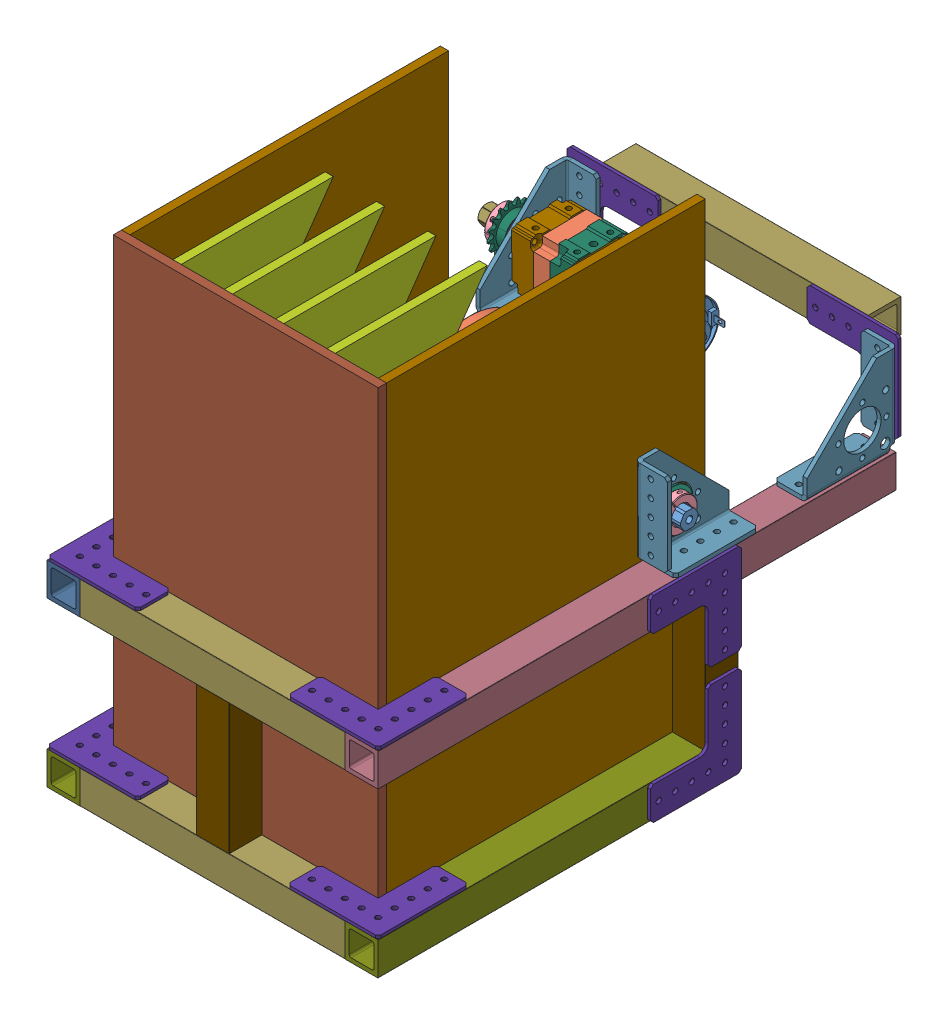
SolidWorks assembly Assem_Launch_Component(wheels,hexshaft,motor,etc.)-SP - Copy, configuration Default. Lengths in mm.
Overall size (290.76 381 426.56).
90 component instances, 36 part files, 140 mates.
Components (placement in the parent):
- ThunderHex(.5 11inch)-SP-1: ThunderHex(.5 11inch)-SP [Default] at (-34.4752 190.5 -222.25) x (0 0.015634 -0.999878) z (-1 0 0) size (13.74 12.75 279.4)
- CompliantWheel(4inch 500)SP-1: CompliantWheel(4inch 500)SP [Default] at (-57.548 185.9668 -238.3103) x (0 -0.486399 -0.873737) z (-1 0 0) size (101.6 101.6 25.4)
  - CompliantWheel(4inch 500)SP.STEP-1: CompliantWheel(4inch 500)SP.STEP [Default] at origin size (101.6 101.6 25.4)
    - 4IN Compliant Wheel FINAL Overmold.STEP-1: 4IN Compliant Wheel FINAL Overmold.STEP [Default] at (-16.2374 3.8509 18.652) size (101.6 101.6 25.4)
    - 2in Wheel Intergrated 0500 HEX Hub.STEP-1: 2in Wheel Intergrated 0500 HEX Hub.STEP [Default] at (-16.2374 3.8509 5.952) x (-1 0 0) z (0 0 -1) size (41.91 41.91 25.4)
- CompliantWheel(4inch 500)SP.STEP-1: CompliantWheel(4inch 500)SP.STEP [Default] at (-82.948 195.0332 -206.1897) x (0 0.486399 0.873737) z (-1 0 0) size (101.6 101.6 25.4)
  - 4IN Compliant Wheel FINAL Overmold.STEP-1: 4IN Compliant Wheel FINAL Overmold.STEP [Default] at (-16.2374 3.8509 18.652) size (101.6 101.6 25.4)
  - 2in Wheel Intergrated 0500 HEX Hub.STEP-1: 2in Wheel Intergrated 0500 HEX Hub.STEP [Default] at (-16.2374 3.8509 5.952) x (-1 0 0) z (0 0 -1) size (41.91 41.91 25.4)
- CompliantWheel(4inch 500)SP.STEP-3: CompliantWheel(4inch 500)SP.STEP [Default] at (-108.348 195.2838 -206.2625) x (0 0.5 0.866025) z (-1 0 0) size (101.6 101.6 25.4)
  - 4IN Compliant Wheel FINAL Overmold.STEP-1: 4IN Compliant Wheel FINAL Overmold.STEP [Default] at (-16.2374 3.8509 18.652) size (101.6 101.6 25.4)
  - 2in Wheel Intergrated 0500 HEX Hub.STEP-1: 2in Wheel Intergrated 0500 HEX Hub.STEP [Default] at (-16.2374 3.8509 5.952) x (-1 0 0) z (0 0 -1) size (41.91 41.91 25.4)
- CompliantWheel(4inch 500)SP.STEP-4: CompliantWheel(4inch 500)SP.STEP [Default] at (-133.748 195.0332 -206.1897) x (0 0.486399 0.873737) z (-1 0 0) size (101.6 101.6 25.4)
  - 4IN Compliant Wheel FINAL Overmold.STEP-1: 4IN Compliant Wheel FINAL Overmold.STEP [Default] at (-16.2374 3.8509 18.652) size (101.6 101.6 25.4)
  - 2in Wheel Intergrated 0500 HEX Hub.STEP-1: 2in Wheel Intergrated 0500 HEX Hub.STEP [Default] at (-16.2374 3.8509 5.952) x (-1 0 0) z (0 0 -1) size (41.91 41.91 25.4)
- ClampingShaftCollar(.5 in)SP-1: ClampingShaftCollar(.5 in)SP [Default] at (-47.625 190.7032 -222.2468) x (0 0.015634 -0.999878) z (-1 0 0) size (25.39 25.4 6.35)
- ClampingShaftCollar(.5 in)SP-2: ClampingShaftCollar(.5 in)SP [Default] at (-155.575 190.4012 -222.4275) x (0 0.873737 -0.486399) z (-1 0 0) size (25.39 25.4 6.35)
- VersaPlanetaryv2_Single_Stage_10_1_with_775_Series (General_GearBox_Shell)-SP-1: VersaPlanetaryv2_Single_Stage_10_1_with_775_Series (General_GearBox_Shell)-SP [Default] at (-205.875 214.6824 -345.637) x (-1 0 0) z (0 -0.015634 0.999878) size (166.6 51.28 52.65)
  - VersaPlanetary_v2_Single_Stage_10_1_with_775_Series (General_GearBox_Shell)-SP.STEP-1: VersaPlanetary_v2_Single_Stage_10_1_with_775_Series (General_GearBox_Shell)-SP.STEP [Default] at origin size (166.6 51.28 52.65)
    - 217-2820 Rev1_Public.STEP-1: 217-2820 Rev1_Public.STEP [Default] at (-4.6546 22.225 0) x (0 -0.456494 0.889726) z (-1 0 0) size (39.22 38.88 17.4)
      - 217-2625-100.STEP-1: 217-2625-100.STEP [Default] at origin size (39.22 38.88 12.7)
        - 217-2625-008 Rev1.STEP-1: 217-2625-008 Rev1.STEP [Default] at origin size (34.7 34.7 4.7)
        - 217-2625-010 Rev1.STEP-1: 217-2625-010 Rev1.STEP [Default] at (0 10.193 3.65) x (0.999813 0.019336 0) z (0 0 1) size (4 4 12)
        - 217-2625-010 Rev1.STEP-2: 217-2625-010 Rev1.STEP [Default] at (8.691 -5.3258 3.65) size (4 4 12)
        - 217-2625-010 Rev1.STEP-3: 217-2625-010 Rev1.STEP [Default] at (-8.691 -5.3258 3.65) size (4 4 12)
        - 217-2625-005 Rev1_Planet_Revolving_Follower01.STEP-1: 217-2625-005 Rev1_Planet_Revolving_Follower01.STEP [Default] at (8.691 -5.3258 6.35) x (0.932816 0.360354 0) z (0 0 1) size (16.89 16.89 8)
        - 217-2625-005 Rev1_Planet_Revolving_Follower01.STEP-2: 217-2625-005 Rev1_Planet_Revolving_Follower01.STEP [Default] at (-8.691 -5.3258 6.35) x (-0.932788 -0.360426 0) z (0 0 1) size (16.89 16.89 8)
        - 217-2625-005 Rev1_Planet_Revolving_Follower01.STEP-3: 217-2625-005 Rev1_Planet_Revolving_Follower01.STEP [Default] at (0 10.193 6.35) x (0.893583 0.448898 0) z (0 0 1) size (16.89 16.89 8)
      - 217-2625-007 Rev1_Public.STEP-1: 217-2625-007 Rev1_Public.STEP [Default] at (0 0 6.7) x (0.992772 0.120019 0) z (0 0 1) size (15.27 15.27 12.7)
    - 217-2625-026 Rev1.STEP-1: 217-2625-026 Rev1.STEP [Default] at (-6.5 22.225 0) x (0 -1 0) z (-1 0 0) size (44.45 42 18.12)
    - 217-2742-001 Rev4.STEP-1: 217-2742-001 Rev4.STEP [Default] at (0.2002 22.225 0) x (1 0 0) z (0 -0.092627 0.995701) size (7 28 28)
    - 217-2742-001 Rev4.STEP-2: 217-2742-001 Rev4.STEP [Default] at (8.2002 22.225 0) size (7 28 28)
    - 217-2625-017 Rev1_9714K61.STEP-1: 217-2625-017 Rev1_9714K61.STEP [Default] at (7.42 22.3002 -0.342) x (0 0.56703 0.823697) z (0 -0.823697 0.56703) size (28.51 4.98 27.43)
    - 217-2625-003 Rev1.STEP-1: 217-2625-003 Rev1.STEP [Default] at (7.4478 22.225 0) x (0 -1 0) z (1 0 0) size (17 17 64.11)
    - 217-2625-018 Rev1_98541A410.STEP-1: 217-2625-018 Rev1_98541A410.STEP [Default] at (-0.7046 22.225 0) x (1 0 0) z (0 -0.017452 0.999848) size (1 19.6 17.4)
    - 832-1750-Ring-Gear-Screw_SSA0832-0500ZC.STEP-1: 832-1750-Ring-Gear-Screw_SSA0832-0500ZC.STEP [Default] at (-30.7 4.725 -17.5) x (0 0.997447 0.071411) z (0 -0.071411 0.997447) size (6.73 48.51 6.73)
    - 832-1750-Ring-Gear-Screw_SSA0832-0500ZC.STEP-2: 832-1750-Ring-Gear-Screw_SSA0832-0500ZC.STEP [Default] at (-30.7 39.725 17.5) x (0 0.005929 0.999982) z (0 -0.999982 0.005929) size (6.73 48.51 6.73)
    - 217-2625-025 Rev1.STEP-1: 217-2625-025 Rev1.STEP [Default] at (-23.2 22.225 0) x (0 -1 0) z (-1 0 0) size (44.45 42 18)
    - 217-4649-002 Rev1_SSA0832-0500ZC.STEP-1: 217-4649-002 Rev1_SSA0832-0500ZC.STEP [Default] at (-34.2 4.2645 17.9605) x (0 0.33842 -0.940995) z (0 0.940995 0.33842) size (6.73 16.76 6.73)
    - 217-4649-002 Rev1_SSA0832-0500ZC.STEP-2: 217-4649-002 Rev1_SSA0832-0500ZC.STEP [Default] at (-34.2 40.1855 -17.9605) x (0 -0.308932 -0.951084) z (0 0.951084 -0.308932) size (6.73 16.76 6.73)
    - 217-4649-006 Rev1_SSA0004-008BA.STEP-1: 217-4649-006 Rev1_SSA0004-008BA.STEP [Default] at (-30.7 22.225 14.5) x (0 0.5 -0.866025) z (0 -0.866025 -0.5) size (7 14 7)
    - 217-4649-006 Rev1_SSA0004-008BA.STEP-2: 217-4649-006 Rev1_SSA0004-008BA.STEP [Default] at (-30.7 22.225 -14.5) x (0 -1 0) z (0 0 1) size (7 14 7)
    - 217-2822-002 Rev4.STEP-1: 217-2822-002 Rev4.STEP [Default] at (-32.45 22.225 0) x (0 -1 0) z (-1 0 0) size (42 42 5.3)
    - 217-4347-000 Rev1.STEP-1: 217-4347-000 Rev1.STEP [Default] at (-34.2 22.225 0) x (-1 0 0) z (0 1 0) size (88 44.3 44.3)
    - 217-2816-001 Rev1.STEP-1: 217-2816-001 Rev1.STEP [Default] at (-6.35 22.225 0) x (0 -1 0) z (1 0 0) size (42 42 14.51)
    - 217-4649-001 Rev1.STEP-1: 217-4649-001 Rev1.STEP [Default] at (-20.554 22.225 0) x (0 -1 0) z (1 0 0) size (18 18 13)
    - 217-4649-007 Rev1_94105A824.STEP-1: 217-4649-007 Rev1_94105A824.STEP [Default] at (-26.029 22.225 -6.7835) x (-0.996104 -0.088191 0) z (0 0 -1) size (4.83 4.83 4.77)
    - 217-2625-013 Rev2.STEP-1: 217-2625-013 Rev2.STEP [Default] at (-25.2898 22.225 0) x (0 0 1) z (-1 0 0) size (8.01 7.94 7.5)
- 13_75mm_1_2_ThunderHex_ID_x_1_125_OD_x_0_313_WD_Flanged_Bearing_217-4006.step-1: 13_75mm_1_2_ThunderHex_ID_x_1_125_OD_x_0_313_WD_Flanged_Bearing_217-4006.step [Default] at (-0.3489 190.5 -222.25) x (0 -0.574166 -0.818739) z (1 0 0) size (31.12 31.12 7.94)
- betterRamp RC-1: betterRamp RC [Default] at (-39.37 168.0882 -127) x (-1 0 0) z (0 0 -1) size (6.35 381 215.9)
- betterRamp RC-2: betterRamp RC [Default] at (-118.11 168.0882 -127) x (-1 0 0) z (0 0 -1) size (6.35 381 215.9)
- betterRamp RC-3: betterRamp RC [Default] at (-78.74 168.0882 -127) x (-1 0 0) z (0 0 -1) size (6.35 381 215.9)
- betterRamp RC-4: betterRamp RC [Default] at (-157.48 168.0882 -127) x (-1 0 0) z (0 0 -1) size (6.35 381 215.9)
- ClampingShaftCollar(.5 in)SP-3: ClampingShaftCollar(.5 in)SP [Default] at (6.9517 190.5 -222.25) x (0 0.858103 0.513478) z (-1 0 0) size (25.39 25.4 6.35)
- ThunderHexFlangedBearing(0.5in) RC-1: ThunderHexFlangedBearing(0.5in) RC [Default] at (-203.9473 190.5 -222.25) x (0 0.030565 0.999533) z (-1 0 0) size (31.12 31.12 7.94)
- ClampingShaftCollar(.5 in)SP-4: ClampingShaftCollar(.5 in)SP [Default] at (-209.7506 190.5 -222.25) x (0 -0.581767 0.813355) z (-1 0 0) size (25.39 25.4 6.35)
- Wall(15 by 15 in .125thickness)-SP-2: Wall(15 by 15 in .125thickness)-SP [Default] at (0 190.5 -128.5875) x (-1 0 0) z (0 0 -1) size (6.35 381 244.47)
- Wall(15 by 15 in .125thickness)-SP-3: Wall(15 by 15 in .125thickness)-SP [Default] at (-203.2 190.5 -128.5875) x (1 0 0) z (0 0 -1) size (6.35 381 244.47)
- 1x1AluminumStock(15in)-1: 1x1AluminumStock(15in) [Default] at (-228.6 139.7 -1803.4) size (25.4 25.4 419.1)
- BackWall-SP-1: BackWall-SP [Default] at (311.6896 672.1897 -6.35) size (203.2 381 6.35)
- 1x1AluminumStock(9.5in)-1: 1x1AluminumStock(9.5in) [Default] at (1625.6 139.7 0) x (0 0 1) z (-1 0 0) size (25.4 25.4 203.2)
- 1x1AluminumStock(9.5in)-2: 1x1AluminumStock(9.5in) [Default] at (1625.6 215.773 -401.0306) x (0 0 1) z (-1 0 0) size (25.4 25.4 203.2)
- 1x1AluminumStock(11in)-2: 1x1AluminumStock(11in) [Default] at (25.4 139.7 1457.1726) x (-1 0 0) z (0 0 -1) size (25.4 25.4 397.03)
- CornerGussetBearingAssem-2: CornerGussetBearingAssem [Default] at (-276.5029 188.5569 -375.7969) x (0 1 0) z (1 0 0) size (69.72 69.72 26.99)
  - CornerGusset-1: CornerGusset [Default] at (-23.4569 2.4523 47.9029) size (69.72 69.72 25.4)
  - ThunderHexFlangedBearing(0.5in) RC-1: ThunderHexFlangedBearing(0.5in) RC [Default] at (3.9032 29.8124 50.2842) x (0.923728 0.383049 0) z (0 0 -1) size (31.12 31.12 7.94)
- 16AluminumSprocket(#25,0.5inHexBore)-1: 16AluminumSprocket(#25,0.5inHexBore) [Default] at (-242.9193 192.4727 -345.9769) x (0 0.486399 0.873737) z (-1 0 0) size (35.22 35.22 9.18)
- 16AluminumSprocket(#25,0.5inHexBore)-2: 16AluminumSprocket(#25,0.5inHexBore) [Default] at (-242.9193 190.5254 -222.2496) x (0 -0.486399 -0.873737) z (-1 0 0) size (35.22 35.22 9.18)
- ClampingShaftCollar(.5 in)SP-5: ClampingShaftCollar(.5 in)SP [Default] at (-233.3625 192.3343 -346.0598) x (0 -0.015634 0.999878) z (-1 0 0) size (25.39 25.4 6.35)
- 1x1AluminumStock(10.88in)-1: 1x1AluminumStock(10.88in) [Default] at (-228.6 14.2875 -1803.273) size (25.4 25.4 276.35)
- 1x1AluminumStock(10.88in)-2: 1x1AluminumStock(10.88in) [Default] at (0 14.2875 -1803.273) size (25.4 25.4 276.35)
- 1x1AluminumStock(9.5in)-3: 1x1AluminumStock(9.5in) [Default] at (1625.6 14.2875 0.127) x (0 0 1) z (-1 0 0) size (25.4 25.4 203.2)
- ClampingShaftCollar(.5 in)SP-6: ClampingShaftCollar(.5 in)SP [Default] at (-233.3625 190.3975 -222.1929) x (0 0.015634 -0.999878) z (1 0 0) size (25.39 25.4 6.35)
- ClampingShaftCollar(.5 in)SP-7: ClampingShaftCollar(.5 in)SP [Default] at (-248.8882 190.3993 -222.3102) x (0 -0.015634 0.999878) z (-1 0 0) size (25.39 25.4 6.35)
- ClampingShaftCollar(.5 in)SP-8: ClampingShaftCollar(.5 in)SP [Default] at (-248.8882 192.332 -345.9131) x (0 -0.015634 0.999878) z (-1 0 0) size (25.39 25.4 6.35)
- L-Bracket(90degree)-2: L-Bracket(90degree) [Default] at (-216.027 167.386 12.827) x (1 0 0) z (0 -1 0) size (69.6 69.6 2.29)
- L-Bracket(90degree)-4: L-Bracket(90degree) [Default] at (12.827 39.6875 12.954) x (-1 0 0) z (0 1 0) size (69.6 69.6 2.29)
- L-Bracket(90degree)-5: L-Bracket(90degree) [Default] at (12.827 165.1 12.827) x (-1 0 0) z (0 1 0) size (69.6 69.6 2.29)
- L-Bracket(90degree)-6: L-Bracket(90degree) [Default] at (-216.027 41.9735 12.954) x (1 0 0) z (0 -1 0) size (69.6 69.6 2.29)
- 1x1AluminumStock(3.95in)-1: 1x1AluminumStock(3.95in) [Default] at (-228.6 1868.4875 -250.825) x (1 0 0) z (0 -1 0) size (25.4 25.4 100.08)
- 1x1AluminumStock(3.95in)-2: 1x1AluminumStock(3.95in) [Default] at (0 1868.4875 -250.825) x (1 0 0) z (0 -1 0) size (25.4 25.4 100.08)
- 1x1AluminumStock(3.95in)-3: 1x1AluminumStock(3.95in) [Default] at (-114.3 1868.4875 0) x (1 0 0) z (0 -1 0) size (25.4 25.4 100.08)
- L-Bracket(90degree)-7: L-Bracket(90degree) [Default] at (25.4 26.8605 -238.252) x (0 0 1) z (1 0 0) size (69.6 69.6 2.29)
- L-Bracket(90degree)-8: L-Bracket(90degree) [Default] at (-230.886 26.8605 -238.252) x (0 0 1) z (1 0 0) size (69.6 69.6 2.29)
- L-Bracket(90degree)-9: L-Bracket(90degree) [Default] at (25.4 152.527 -238.252) x (0 -1 0) z (1 0 0) size (69.6 69.6 2.29)
- L-Bracket(90degree)-10: L-Bracket(90degree) [Default] at (-230.886 152.527 -238.252) x (0 -1 0) z (1 0 0) size (69.6 69.6 2.29)
- CornerGusset-1: CornerGusset [Default] at (0 165.1 -196.2958) x (0 0 -1) z (1 0 0) size (69.72 69.72 25.4)
- CornerGusset-2: CornerGusset [Default] at (-203.2 165.1 -195.1148) x (0 1 0) z (-1 0 0) size (69.72 69.72 25.4)
- CornerGusset-3: CornerGusset [Default] at (25.4 165.1 -373.3446) x (0 0 1) z (-1 0 0) size (69.72 69.72 25.4)
- L-Bracket(90degree)-11: L-Bracket(90degree) [Default] at (12.7 228.6 -375.6306) x (0 -1 0) z (0 0 1) size (69.6 69.6 2.29)
- L-Bracket(90degree)-12: L-Bracket(90degree) [Default] at (-215.9 228.6 -375.6306) size (69.6 69.6 2.29)
Mates (geometry in assembly coordinates):
- Coincident1: coincident: plane of ThunderHex(.5 11inch)-SP-1 through (-263.0752 184.0678 -218.6693) normal (0 -0.513478 0.858103); plane of CompliantWheel(4inch 500)SP-1/CompliantWheel(4inch 500)SP.STEP-1/2in Wheel Intergrated 0500 HEX Hub.STEP-1 through (-50.8 184.0678 -218.6693) normal (0 0.513478 -0.858103)
- Coincident2: coincident: plane of ThunderHex(.5 11inch)-SP-1 through (-263.0752 184.1829 -226.0301) normal (0 -0.999878 -0.015634); plane of CompliantWheel(4inch 500)SP-1/CompliantWheel(4inch 500)SP.STEP-1/2in Wheel Intergrated 0500 HEX Hub.STEP-1 through (-50.8 184.1829 -226.0301) normal (0 0.999878 0.015634)
- Coincident3: coincident: circle of CompliantWheel(4inch 500)SP-1/CompliantWheel(4inch 500)SP.STEP-1/2in Wheel Intergrated 0500 HEX Hub.STEP-1; plane of CompliantWheel(4inch 500)SP.STEP-1/2in Wheel Intergrated 0500 HEX Hub.STEP-1 through (-76.2 192.7193 -223.4855) normal (1 0 0)
- Coincident5: coincident: circle of CompliantWheel(4inch 500)SP.STEP-3/2in Wheel Intergrated 0500 HEX Hub.STEP-1; plane of CompliantWheel(4inch 500)SP.STEP-4/2in Wheel Intergrated 0500 HEX Hub.STEP-1 through (-127 192.7193 -223.4855) normal (1 0 0)
- Coincident7: coincident: plane of CompliantWheel(4inch 500)SP-1/CompliantWheel(4inch 500)SP.STEP-1/2in Wheel Intergrated 0500 HEX Hub.STEP-1 through (-50.8 188.2807 -221.0145) normal (1 0 0); plane of ClampingShaftCollar(.5 in)SP-1 through (-50.8 190.7032 -222.2468) normal (-1 0 0)
- Coincident8: coincident: plane of ThunderHex(.5 11inch)-SP-1 through (-263.0752 184.0678 -218.6693) normal (0 -0.513478 0.858103); plane of ClampingShaftCollar(.5 in)SP-1 through (-44.45 184.1685 -218.609) normal (0 0.513478 -0.858103)
- Coincident9: coincident: plane of ThunderHex(.5 11inch)-SP-1 through (-263.0752 190.6151 -229.6108) normal (0 -0.486399 -0.873737); plane of ClampingShaftCollar(.5 in)SP-1 through (-44.45 190.8201 -229.7249) normal (0 0.486399 0.873737)
- Coincident13: coincident: plane of CompliantWheel(4inch 500)SP.STEP-4/2in Wheel Intergrated 0500 HEX Hub.STEP-1 through (-152.4 192.7193 -223.4855) normal (-1 0 0); plane of ClampingShaftCollar(.5 in)SP-2 through (-152.4 190.4012 -222.4275) normal (1 0 0)
- Concentric2: concentric: circle of ThunderHex(.5 11inch)-SP-1; circle of 13_75mm_1_2_ThunderHex_ID_x_1_125_OD_x_0_313_WD_Flanged_Bearing_217-4006.step-1
- Concentric4: concentric: circle of CompliantWheel(4inch 500)SP-1/CompliantWheel(4inch 500)SP.STEP-1/4IN Compliant Wheel FINAL Overmold.STEP-1; circle of betterRamp RC-1
- Parallel1: parallel: plane of assembly through (0 0 0) normal (0 1 0); plane of betterRamp RC-1 through (-45.72 0 -222.25) normal (0 -1 0); plane of assembly
- Concentric5: concentric: circle of CompliantWheel(4inch 500)SP-1/CompliantWheel(4inch 500)SP.STEP-1/4IN Compliant Wheel FINAL Overmold.STEP-1; circle of betterRamp RC-2
- Parallel2: parallel: plane of betterRamp RC-1 through (-45.72 0 -222.25) normal (0 -1 0); plane of betterRamp RC-2 through (-124.46 0 -222.25) normal (0 -1 0)
- Concentric6: concentric: circle of CompliantWheel(4inch 500)SP-1/CompliantWheel(4inch 500)SP.STEP-1/4IN Compliant Wheel FINAL Overmold.STEP-1; circle of betterRamp RC-3
- Parallel3: parallel: plane of betterRamp RC-2 through (-124.46 0 -222.25) normal (0 -1 0); plane of betterRamp RC-3 through (-85.09 0 -222.25) normal (0 -1 0)
- Concentric7: concentric: circle of CompliantWheel(4inch 500)SP-1/CompliantWheel(4inch 500)SP.STEP-1/4IN Compliant Wheel FINAL Overmold.STEP-1; circle of betterRamp RC-4
- Parallel4: parallel: plane of betterRamp RC-2 through (-124.46 0 -222.25) normal (0 -1 0); plane of betterRamp RC-4 through (-163.83 0 -222.25) normal (0 -1 0)
- Concentric8: concentric: circle of ThunderHex(.5 11inch)-SP-1; circle of ClampingShaftCollar(.5 in)SP-3
- Parallel5: parallel: plane of ThunderHex(.5 11inch)-SP-1 through (-263.0752 184.0678 -218.6693) normal (0 -0.513478 0.858103); plane of ClampingShaftCollar(.5 in)SP-3 through (10.1267 197.0347 -225.8878) normal (0 -0.513478 0.858103)
- Concentric9: concentric: circle of ThunderHex(.5 11inch)-SP-1; circle of ThunderHexFlangedBearing(0.5in) RC-1
- Concentric10: concentric: circle of ThunderHex(.5 11inch)-SP-1; circle of ClampingShaftCollar(.5 in)SP-4
- Concentric12: concentric: circle of 13_75mm_1_2_ThunderHex_ID_x_1_125_OD_x_0_313_WD_Flanged_Bearing_217-4006.step-1; circle of Wall(15 by 15 in .125thickness)-SP-2
- Concentric15: concentric: circle of Wall(15 by 15 in .125thickness)-SP-2; circle of Wall(15 by 15 in .125thickness)-SP-3
- Parallel7: parallel: plane of betterRamp RC-1 through (-45.72 0 -222.25) normal (0 -1 0); plane of Wall(15 by 15 in .125thickness)-SP-2 through (-6.35 0 -6.35) normal (0 -1 0)
- Distance13: distance = 44.45 mm: plane of Wall(15 by 15 in .125thickness)-SP-2 through (-6.35 190.5 -128.5875) normal (-1 0 0); plane of CompliantWheel(4inch 500)SP-1/CompliantWheel(4inch 500)SP.STEP-1/4IN Compliant Wheel FINAL Overmold.STEP-1 through (-50.8 168.1398 -209.8023) normal (1 0 0)
- Distance14: distance = 44.45 mm: plane of CompliantWheel(4inch 500)SP.STEP-4/4IN Compliant Wheel FINAL Overmold.STEP-1 through (-152.4 208.4217 -232.2268) normal (-1 0 0); plane of Wall(15 by 15 in .125thickness)-SP-3 through (-196.85 190.5 -128.5875) normal (1 0 0)
- Parallel14: parallel: plane of betterRamp RC-4 through (-163.83 0 -6.35) normal (0 0 1); plane of Wall(15 by 15 in .125thickness)-SP-3 through (-196.85 0 -6.35) normal (0 0 1)
- Distance15: distance = 190.5 mm: plane of Wall(15 by 15 in .125thickness)-SP-3 through (-196.85 190.5 -128.5875) normal (1 0 0); plane of Wall(15 by 15 in .125thickness)-SP-2 through (-6.35 190.5 -128.5875) normal (-1 0 0)
- Distance16: distance = 33.02 mm: plane of Wall(15 by 15 in .125thickness)-SP-2 through (-6.35 190.5 -128.5875) normal (-1 0 0); plane of betterRamp RC-1 through (-39.37 168.0882 -127) normal (1 0 0)
- Concentric16: concentric: circle of CompliantWheel(4inch 500)SP-1/CompliantWheel(4inch 500)SP.STEP-1/4IN Compliant Wheel FINAL Overmold.STEP-1; circle of CompliantWheel(4inch 500)SP.STEP-1/4IN Compliant Wheel FINAL Overmold.STEP-1
- Distance18: distance = 33.02 mm: plane of betterRamp RC-3 through (-85.09 168.0882 -127) normal (-1 0 0); plane of betterRamp RC-2 through (-118.11 168.0882 -127) normal (1 0 0)
- Distance19: distance = 33.02 mm: plane of betterRamp RC-4 through (-157.48 168.0882 -127) normal (1 0 0); plane of betterRamp RC-2 through (-124.46 168.0882 -127) normal (-1 0 0)
- Coincident50: coincident: line of betterRamp RC-3 through (-85.09 381 -6.35) axis (1 0 0); line of BackWall-SP-1 through (0 381 -6.35) axis (-1 0 0)
- Coincident51: coincident: line of Wall(15 by 15 in .125thickness)-SP-2 through (0 0 -6.35) axis (0 1 0); line of BackWall-SP-1 through (0 0 -6.35) axis (0 1 0)
- Coincident53: coincident: plane of Wall(15 by 15 in .125thickness)-SP-3 through (-203.2 190.5 -128.5875) normal (-1 0 0); plane of 1x1AluminumStock(15in)-1 through (-203.2 139.954 25.4) normal (1 0 0)
- Coincident67: coincident: plane of BackWall-SP-1 through (311.6896 672.1897 0) normal (0 0 1); plane of 1x1AluminumStock(9.5in)-1 through (-203.2 139.954 0) normal (0 0 -1)
- Coincident79: coincident: plane of Wall(15 by 15 in .125thickness)-SP-2 through (0 190.5 -128.5875) normal (1 0 0); plane of 1x1AluminumStock(11in)-2 through (0 139.954 -371.6274) normal (-1 0 0)
- Coincident80: coincident: plane of 1x1AluminumStock(9.5in)-1 through (-203.2 139.954 25.4) normal (0 0 1); plane of 1x1AluminumStock(11in)-2 through (0 586.7809 25.4) normal (0 0 1)
- Coincident81: coincident: plane of 1x1AluminumStock(9.5in)-1 through (-203.2 139.7 0.254) normal (0 -1 0); plane of 1x1AluminumStock(11in)-2 through (25.146 139.7 -371.6274) normal (0 -1 0)
- Concentric17: concentric: circle of CompliantWheel(4inch 500)SP.STEP-1/4IN Compliant Wheel FINAL Overmold.STEP-1; circle of CompliantWheel(4inch 500)SP.STEP-3/4IN Compliant Wheel FINAL Overmold.STEP-1
- Concentric18: concentric: circle of CompliantWheel(4inch 500)SP.STEP-3/4IN Compliant Wheel FINAL Overmold.STEP-1; circle of CompliantWheel(4inch 500)SP.STEP-4/4IN Compliant Wheel FINAL Overmold.STEP-1
- Concentric20: concentric: circle of VersaPlanetaryv2_Single_Stage_10_1_with_775_Series (General_GearBox_Shell)-SP-1/VersaPlanetary_v2_Single_Stage_10_1_with_775_Series (General_GearBox_Shell)-SP.STEP-1/217-2625-003 Rev1.STEP-1; circle of CornerGussetBearingAssem-2/ThunderHexFlangedBearing(0.5in) RC-1
- Parallel15: parallel: plane of ThunderHex(.5 11inch)-SP-1 through (-263.0752 196.8171 -218.4699) normal (0 0.999878 0.015634); plane of VersaPlanetaryv2_Single_Stage_10_1_with_775_Series (General_GearBox_Shell)-SP-1/VersaPlanetary_v2_Single_Stage_10_1_with_775_Series (General_GearBox_Shell)-SP.STEP-1/217-2625-003 Rev1.STEP-1 through (-263.0752 198.752 -342.2195) normal (0 0.999878 0.015634)
- Coincident100: coincident: plane of VersaPlanetaryv2_Single_Stage_10_1_with_775_Series (General_GearBox_Shell)-SP-1/VersaPlanetary_v2_Single_Stage_10_1_with_775_Series (General_GearBox_Shell)-SP.STEP-1/217-2625-026 Rev1.STEP-1 through (-222.5 169.8904 -324.1097) normal (-1 0 0); plane of CornerGussetBearingAssem-2/ThunderHexFlangedBearing(0.5in) RC-1 through (-222.5 196.1382 -354.8541) normal (1 0 0)
- Coincident105: coincident: plane of VersaPlanetaryv2_Single_Stage_10_1_with_775_Series (General_GearBox_Shell)-SP-1/VersaPlanetary_v2_Single_Stage_10_1_with_775_Series (General_GearBox_Shell)-SP.STEP-1/217-2625-003 Rev1.STEP-1 through (-263.0752 186.1682 -349.7495) normal (0 -0.999878 -0.015634); plane of 16AluminumSprocket(#25,0.5inHexBore)-1 through (-236.5365 186.1682 -349.7495) normal (0 0.999878 0.015634)
- Coincident106: coincident: plane of VersaPlanetaryv2_Single_Stage_10_1_with_775_Series (General_GearBox_Shell)-SP-1/VersaPlanetary_v2_Single_Stage_10_1_with_775_Series (General_GearBox_Shell)-SP.STEP-1/217-2625-003 Rev1.STEP-1 through (-263.0752 192.5748 -353.3159) normal (0 -0.486399 -0.873737); plane of 16AluminumSprocket(#25,0.5inHexBore)-1 through (-236.5365 192.5876 -353.3231) normal (0 0.486399 0.873737)
- Coincident108: coincident: plane of ThunderHex(.5 11inch)-SP-1 through (-263.0752 196.9322 -225.8307) normal (0 0.513478 -0.858103); plane of 16AluminumSprocket(#25,0.5inHexBore)-2 through (-236.5365 196.9448 -225.8232) normal (0 -0.513478 0.858103)
- Coincident109: coincident: plane of ThunderHex(.5 11inch)-SP-1 through (-263.0752 190.3849 -214.8892) normal (0 0.486399 0.873737); plane of 16AluminumSprocket(#25,0.5inHexBore)-2 through (-236.5365 190.4105 -214.9035) normal (0 -0.486399 -0.873737)
- Coincident110: coincident: plane of 16AluminumSprocket(#25,0.5inHexBore)-1 through (-245.7132 192.4727 -345.9769) normal (-1 0 0); plane of 16AluminumSprocket(#25,0.5inHexBore)-2 through (-245.7132 190.5254 -222.2496) normal (-1 0 0)
- Coincident111: coincident: point of assembly; point of BackWall-SP-1; point of assembly
- Coincident112: coincident: plane of ThunderHex(.5 11inch)-SP-1 through (-263.0752 184.0678 -218.6693) normal (0 -0.513478 0.858103); plane of ClampingShaftCollar(.5 in)SP-2 through (-152.4 183.8665 -218.7898) normal (0 0.513478 -0.858103)
- Coincident113: coincident: plane of ThunderHex(.5 11inch)-SP-1 through (-263.0752 196.8171 -218.4699) normal (0 0.999878 0.015634); plane of ClampingShaftCollar(.5 in)SP-2 through (-152.4 196.8189 -218.5872) normal (0 -0.999878 -0.015634)
- Coincident116: coincident: plane of assembly through (0 0 0) normal (0 1 0); plane of BackWall-SP-1 through (-203.2 0 0) normal (0 -1 0); plane of assembly
- Coincident120: coincident: plane of 1x1AluminumStock(15in)-1 through (-228.346 165.1 25.4) normal (0 1 0); plane of 1x1AluminumStock(9.5in)-1 through (-203.2 165.1 0.254) normal (0 1 0)
- Coincident121: coincident: plane of Wall(15 by 15 in .125thickness)-SP-3 through (-203.2 190.5 -128.5875) normal (-1 0 0); plane of 1x1AluminumStock(15in)-1 through (-203.2 139.954 25.4) normal (1 0 0)
- Coincident122: coincident: plane of 1x1AluminumStock(15in)-1 through (-228.346 139.954 25.4) normal (0 0 1); plane of 1x1AluminumStock(9.5in)-1 through (-203.2 139.954 25.4) normal (0 0 1)
- Coincident123: coincident: plane of 1x1AluminumStock(15in)-1 through (-203.2 139.954 25.4) normal (1 0 0); plane of 1x1AluminumStock(9.5in)-1 through (-203.2 139.954 0.254) normal (-1 0 0)
- Coincident124: coincident: plane of 1x1AluminumStock(15in)-1 through (-228.346 165.1 25.4) normal (0 1 0); plane of CornerGussetBearingAssem-2/CornerGusset-1 through (-228.6 165.1 -373.3446) normal (0 -1 0)
- Coincident129: coincident: plane of ThunderHex(.5 11inch)-SP-1 through (-263.0752 196.8171 -218.4699) normal (0 0.999878 0.015634); plane of VersaPlanetaryv2_Single_Stage_10_1_with_775_Series (General_GearBox_Shell)-SP-1/VersaPlanetary_v2_Single_Stage_10_1_with_775_Series (General_GearBox_Shell)-SP.STEP-1/217-2625-003 Rev1.STEP-1 through (-263.0752 198.752 -342.2195) normal (0 0.999878 0.015634)
- Parallel19: parallel: plane of assembly through (0 0 0) normal (1 0 0); plane of betterRamp RC-1 through (-39.37 168.0882 -127) normal (1 0 0); plane of assembly
- Parallel21: parallel: plane of 1x1AluminumStock(9.5in)-2 through (0 662.8539 -375.6306) normal (1 0 0); plane of 1x1AluminumStock(11in)-2 through (0 139.954 -371.6274) normal (-1 0 0)
- Distance28: distance = 33.02 mm: plane of betterRamp RC-3 through (-78.74 168.0882 -127) normal (1 0 0); plane of betterRamp RC-1 through (-45.72 168.0882 -127) normal (-1 0 0)
- Distance31: distance = 139.7 mm: plane of 1x1AluminumStock(11in)-2 through (25.146 139.7 -371.6274) normal (0 -1 0); plane of Wall(15 by 15 in .125thickness)-SP-2 through (-6.35 0 -6.35) normal (0 -1 0)
- Coincident141: coincident: unknown of CompliantWheel(4inch 500)SP-1/CompliantWheel(4inch 500)SP.STEP-1/4IN Compliant Wheel FINAL Overmold.STEP-1; line of CompliantWheel(4inch 500)SP.STEP-1/4IN Compliant Wheel FINAL Overmold.STEP-1 through (-101.346 165.7909 -266.6358) axis (1 0 0)
- Coincident142: coincident: line of CompliantWheel(4inch 500)SP.STEP-1/4IN Compliant Wheel FINAL Overmold.STEP-1 through (-101.346 165.7909 -266.6358) axis (1 0 0); line of CompliantWheel(4inch 500)SP.STEP-4/4IN Compliant Wheel FINAL Overmold.STEP-1 through (-152.146 165.7909 -266.6358) axis (1 0 0)
- Distance35: distance = 50.8 mm: cylinder of VersaPlanetaryv2_Single_Stage_10_1_with_775_Series (General_GearBox_Shell)-SP-1/VersaPlanetary_v2_Single_Stage_10_1_with_775_Series (General_GearBox_Shell)-SP.STEP-1/217-4347-000 Rev1.STEP-1 through (-107.8028 192.4601 -345.9845) axis (1 0 0) radius 22.15; cylinder of CompliantWheel(4inch 500)SP.STEP-4/4IN Compliant Wheel FINAL Overmold.STEP-1 through (-182.1962 190.5 -222.25) axis (1 0 0) radius 50.8
- Coincident155: coincident: plane of Wall(15 by 15 in .125thickness)-SP-3 through (-203.2 190.5 -128.5875) normal (-1 0 0); plane of 1x1AluminumStock(10.88in)-1 through (-203.2 14.5415 25.527) normal (1 0 0)
- Coincident156: coincident: plane of Wall(15 by 15 in .125thickness)-SP-3 through (-196.85 0 -250.825) normal (0 0 -1); plane of 1x1AluminumStock(10.88in)-1 through (-203.2 461.3684 -250.825) normal (0 0 -1)
- Coincident158: coincident: plane of Wall(15 by 15 in .125thickness)-SP-2 through (0 190.5 -128.5875) normal (1 0 0); plane of 1x1AluminumStock(10.88in)-2 through (0 14.5415 25.527) normal (-1 0 0)
- Coincident159: coincident: plane of Wall(15 by 15 in .125thickness)-SP-2 through (-6.35 381 -250.825) normal (0 0 -1); plane of 1x1AluminumStock(10.88in)-2 through (25.4 461.3684 -250.825) normal (0 0 -1)
- Coincident161: coincident: plane of 1x1AluminumStock(10.88in)-1 through (-203.2 14.5415 25.527) normal (1 0 0); plane of 1x1AluminumStock(9.5in)-3 through (-203.2 14.5415 0.381) normal (-1 0 0)
- Coincident162: coincident: plane of 1x1AluminumStock(10.88in)-1 through (-228.346 14.5415 25.527) normal (0 0 1); plane of 1x1AluminumStock(9.5in)-3 through (-203.2 14.5415 25.527) normal (0 0 1)
- Coincident163: coincident: plane of 1x1AluminumStock(10.88in)-1 through (-228.346 39.6875 25.527) normal (0 1 0); plane of 1x1AluminumStock(9.5in)-3 through (-203.2 39.6875 0.381) normal (0 1 0)
- Coincident164: coincident: plane of 1x1AluminumStock(15in)-1 through (-203.2 139.954 25.4) normal (1 0 0); plane of CornerGussetBearingAssem-2/CornerGusset-1 through (-203.2 165.1 -303.6216) normal (1 0 0)
- Coincident166: coincident: plane of VersaPlanetaryv2_Single_Stage_10_1_with_775_Series (General_GearBox_Shell)-SP-1/VersaPlanetary_v2_Single_Stage_10_1_with_775_Series (General_GearBox_Shell)-SP.STEP-1/217-2625-003 Rev1.STEP-1 through (-263.0752 198.752 -342.2195) normal (0 0.999878 0.015634); plane of ClampingShaftCollar(.5 in)SP-5 through (-230.1875 198.752 -342.2195) normal (0 -0.999878 -0.015634)
- Coincident167: coincident: plane of VersaPlanetaryv2_Single_Stage_10_1_with_775_Series (General_GearBox_Shell)-SP-1/VersaPlanetary_v2_Single_Stage_10_1_with_775_Series (General_GearBox_Shell)-SP.STEP-1/217-2625-003 Rev1.STEP-1 through (-263.0752 192.3455 -338.653) normal (0 0.486399 0.873737); plane of ClampingShaftCollar(.5 in)SP-5 through (-230.1875 192.2174 -338.5817) normal (0 -0.486399 -0.873737)
- Coincident168: coincident: plane of CornerGussetBearingAssem-2/ThunderHexFlangedBearing(0.5in) RC-1 through (-230.1875 196.1382 -354.8541) normal (-1 0 0); circle of ClampingShaftCollar(.5 in)SP-5
- Coincident170: coincident: plane of 16AluminumSprocket(#25,0.5inHexBore)-1 through (-245.7132 192.4727 -345.9769) normal (-1 0 0); plane of 16AluminumSprocket(#25,0.5inHexBore)-2 through (-245.7132 190.5254 -222.2496) normal (-1 0 0)
- Coincident171: coincident: plane of ThunderHex(.5 11inch)-SP-1 through (-263.0752 190.5 -222.25) normal (-1 0 0); plane of VersaPlanetaryv2_Single_Stage_10_1_with_775_Series (General_GearBox_Shell)-SP-1/VersaPlanetary_v2_Single_Stage_10_1_with_775_Series (General_GearBox_Shell)-SP.STEP-1/217-2625-003 Rev1.STEP-1 through (-263.0752 186.0536 -342.418) normal (-1 0 0)
- Coincident172: coincident: plane of ThunderHex(.5 11inch)-SP-1 through (-263.0752 196.8171 -218.4699) normal (0 0.999878 0.015634); plane of ClampingShaftCollar(.5 in)SP-6 through (-236.5375 196.9322 -225.8307) normal (0 -0.999878 -0.015634)
- Coincident173: coincident: plane of ThunderHex(.5 11inch)-SP-1 through (-263.0752 196.9322 -225.8307) normal (0 0.513478 -0.858103); plane of ClampingShaftCollar(.5 in)SP-6 through (-236.5375 190.5144 -229.671) normal (0 -0.513478 0.858103)
- Coincident175: coincident: plane of ThunderHex(.5 11inch)-SP-1 through (-263.0752 196.8171 -218.4699) normal (0 0.999878 0.015634); plane of ClampingShaftCollar(.5 in)SP-7 through (-245.7132 196.8171 -218.4699) normal (0 -0.999878 -0.015634)
- Coincident176: coincident: plane of ThunderHex(.5 11inch)-SP-1 through (-263.0752 190.3849 -214.8892) normal (0 0.486399 0.873737); plane of ClampingShaftCollar(.5 in)SP-7 through (-245.7132 190.2824 -214.8322) normal (0 -0.486399 -0.873737)
- Coincident177: coincident: plane of 16AluminumSprocket(#25,0.5inHexBore)-2 through (-245.7132 190.5254 -222.2496) normal (-1 0 0); plane of ClampingShaftCollar(.5 in)SP-7 through (-245.7132 190.3993 -222.3102) normal (1 0 0)
- Coincident182: coincident: plane of VersaPlanetaryv2_Single_Stage_10_1_with_775_Series (General_GearBox_Shell)-SP-1/VersaPlanetary_v2_Single_Stage_10_1_with_775_Series (General_GearBox_Shell)-SP.STEP-1/217-2625-003 Rev1.STEP-1 through (-263.0752 198.752 -342.2195) normal (0 0.999878 0.015634); plane of ClampingShaftCollar(.5 in)SP-8 through (-245.7132 198.7497 -342.0728) normal (0 -0.999878 -0.015634)
- Coincident184: coincident: plane of VersaPlanetaryv2_Single_Stage_10_1_with_775_Series (General_GearBox_Shell)-SP-1/VersaPlanetary_v2_Single_Stage_10_1_with_775_Series (General_GearBox_Shell)-SP.STEP-1/217-2625-003 Rev1.STEP-1 through (-263.0752 198.8667 -349.5509) normal (0 0.513478 -0.858103); plane of ClampingShaftCollar(.5 in)SP-8 through (-245.7132 198.8667 -349.5509) normal (0 -0.513478 0.858103)
- Coincident185: coincident: plane of 16AluminumSprocket(#25,0.5inHexBore)-1 through (-245.7132 192.4727 -345.9769) normal (-1 0 0); plane of ClampingShaftCollar(.5 in)SP-8 through (-245.7132 192.332 -345.9131) normal (1 0 0)
- Coincident186: coincident: plane of 16AluminumSprocket(#25,0.5inHexBore)-1 through (-236.5375 192.4727 -345.9769) normal (1 0 0); plane of ClampingShaftCollar(.5 in)SP-5 through (-236.5375 192.3343 -346.0598) normal (-1 0 0)
- Coincident190: coincident: plane of 1x1AluminumStock(11in)-2 through (25.146 165.1 -371.6274) normal (0 1 0); plane of L-Bracket(90degree)-5 through (25.4 165.1 25.4) normal (0 -1 0)
- Coincident191: coincident: plane of 1x1AluminumStock(11in)-2 through (25.4 139.954 -371.6274) normal (1 0 0); plane of L-Bracket(90degree)-5 through (25.4 167.386 -44.196) normal (1 0 0)
- Coincident192: coincident: plane of 1x1AluminumStock(11in)-2 through (0 586.7809 25.4) normal (0 0 1); plane of L-Bracket(90degree)-5 through (25.4 167.386 25.4) normal (0 0 1)
- Coincident199: coincident: plane of 1x1AluminumStock(15in)-1 through (-228.346 165.1 25.4) normal (0 1 0); plane of L-Bracket(90degree)-2 through (-228.6 165.1 25.4) normal (0 -1 0)
- Coincident200: coincident: plane of 1x1AluminumStock(15in)-1 through (-228.6 139.954 25.4) normal (-1 0 0); plane of L-Bracket(90degree)-2 through (-228.6 165.1 -44.196) normal (-1 0 0)
- Coincident201: coincident: plane of 1x1AluminumStock(15in)-1 through (-228.346 139.954 25.4) normal (0 0 1); plane of L-Bracket(90degree)-2 through (-228.6 165.1 25.4) normal (0 0 1)
- Coincident202: coincident: plane of 1x1AluminumStock(10.88in)-2 through (0.254 39.6875 25.527) normal (0 1 0); plane of L-Bracket(90degree)-4 through (25.4 39.6875 25.527) normal (0 -1 0)
- Coincident203: coincident: plane of 1x1AluminumStock(10.88in)-2 through (0.254 14.5415 25.527) normal (0 0 1); plane of L-Bracket(90degree)-4 through (25.4 41.9735 25.527) normal (0 0 1)
- Coincident204: coincident: plane of 1x1AluminumStock(10.88in)-2 through (25.4 14.5415 25.527) normal (1 0 0); plane of L-Bracket(90degree)-4 through (25.4 41.9735 -44.069) normal (1 0 0)
- Coincident207: coincident: plane of 1x1AluminumStock(10.88in)-1 through (-228.6 14.5415 25.527) normal (-1 0 0); plane of L-Bracket(90degree)-6 through (-228.6 39.6875 -44.069) normal (-1 0 0)
- Coincident208: coincident: plane of 1x1AluminumStock(10.88in)-1 through (-228.346 39.6875 25.527) normal (0 1 0); plane of L-Bracket(90degree)-6 through (-228.6 39.6875 25.527) normal (0 -1 0)
- Coincident209: coincident: plane of 1x1AluminumStock(10.88in)-1 through (-228.346 14.5415 25.527) normal (0 0 1); plane of L-Bracket(90degree)-6 through (-228.6 39.6875 25.527) normal (0 0 1)
- Concentric21: concentric: cylinder of ThunderHex(.5 11inch)-SP-1 through (194.1248 190.5 -222.25) axis (-1 0 0) radius 2.55; cylinder of betterRamp RC-1 through (-39.37 190.5 -222.25) axis (-1 0 0) radius 190.5
- Distance38: distance = 14.2875 mm: plane of Wall(15 by 15 in .125thickness)-SP-2 through (-6.35 0 -6.35) normal (0 -1 0); plane of 1x1AluminumStock(10.88in)-2 through (0.254 14.2875 25.527) normal (0 -1 0)
- Coincident214: coincident: plane of 1x1AluminumStock(9.5in)-3 through (-203.2 39.6875 0.381) normal (0 1 0); plane of L-Bracket(90degree)-4 through (25.4 39.6875 25.527) normal (0 -1 0)
- Coincident215: coincident: plane of 1x1AluminumStock(10.88in)-1 through (-228.346 39.6875 25.527) normal (0 1 0); plane of 1x1AluminumStock(3.95in)-1 through (-228.346 39.6875 -250.571) normal (0 -1 0)
- Coincident216: coincident: plane of Wall(15 by 15 in .125thickness)-SP-3 through (-203.2 190.5 -128.5875) normal (-1 0 0); plane of 1x1AluminumStock(3.95in)-1 through (-203.2 39.6875 -250.571) normal (1 0 0)
- Coincident217: coincident: line of 1x1AluminumStock(10.88in)-1 through (-228.346 39.6875 -250.825) axis (1 0 0); line of 1x1AluminumStock(3.95in)-1 through (-228.346 39.6875 -250.825) axis (1 0 0)
- Coincident218: coincident: plane of Wall(15 by 15 in .125thickness)-SP-2 through (0 190.5 -128.5875) normal (1 0 0); plane of 1x1AluminumStock(3.95in)-2 through (0 39.6875 -250.571) normal (-1 0 0)
- Coincident219: coincident: plane of 1x1AluminumStock(10.88in)-2 through (0.254 39.6875 25.527) normal (0 1 0); plane of 1x1AluminumStock(3.95in)-2 through (0.254 39.6875 -250.571) normal (0 -1 0)
- Coincident220: coincident: line of 1x1AluminumStock(10.88in)-2 through (0.254 39.6875 -250.825) axis (1 0 0); line of 1x1AluminumStock(3.95in)-2 through (0.254 39.6875 -250.825) axis (1 0 0)
- Distance40: distance = 114.3 mm: plane of 1x1AluminumStock(3.95in)-3 through (-114.3 39.6875 0.254) normal (-1 0 0); plane of 1x1AluminumStock(10.88in)-1 through (-228.6 14.5415 25.527) normal (-1 0 0)
- Coincident222: coincident: plane of 1x1AluminumStock(9.5in)-3 through (-203.2 39.6875 0.381) normal (0 1 0); plane of 1x1AluminumStock(3.95in)-3 through (-114.046 39.6875 0.254) normal (0 -1 0)
- Coincident223: coincident: plane of BackWall-SP-1 through (311.6896 672.1897 0) normal (0 0 1); plane of 1x1AluminumStock(3.95in)-3 through (-114.046 39.6875 0) normal (0 0 -1)
- Coincident224: coincident: plane of 1x1AluminumStock(10.88in)-2 through (25.4 14.5415 25.527) normal (1 0 0); plane of L-Bracket(90degree)-7 through (25.4 14.2875 -250.825) normal (-1 0 0)
- Coincident225: coincident: plane of 1x1AluminumStock(3.95in)-2 through (0.254 39.6875 -250.825) normal (0 0 -1); plane of L-Bracket(90degree)-7 through (27.686 83.8835 -250.825) normal (0 0 -1)
- Coincident226: coincident: plane of 1x1AluminumStock(10.88in)-2 through (0.254 14.2875 25.527) normal (0 -1 0); plane of L-Bracket(90degree)-7 through (27.686 14.2875 -250.825) normal (0 -1 0)
- Coincident227: coincident: plane of 1x1AluminumStock(10.88in)-1 through (-228.6 14.5415 25.527) normal (-1 0 0); plane of L-Bracket(90degree)-8 through (-228.6 14.2875 -250.825) normal (1 0 0)
- Coincident228: coincident: plane of 1x1AluminumStock(10.88in)-1 through (-228.346 14.2875 25.527) normal (0 -1 0); plane of L-Bracket(90degree)-8 through (-228.6 14.2875 -250.825) normal (0 -1 0)
- Coincident229: coincident: plane of 1x1AluminumStock(10.88in)-1 through (-203.2 461.3684 -250.825) normal (0 0 -1); plane of L-Bracket(90degree)-8 through (-228.6 83.8835 -250.825) normal (0 0 -1)
- Coincident231: coincident: plane of 1x1AluminumStock(11in)-2 through (25.146 165.1 -371.6274) normal (0 1 0); plane of L-Bracket(90degree)-9 through (27.686 165.1 -181.229) normal (0 1 0)
- Coincident232: coincident: plane of 1x1AluminumStock(3.95in)-2 through (0.254 39.6875 -250.825) normal (0 0 -1); plane of L-Bracket(90degree)-9 through (27.686 165.1 -250.825) normal (0 0 -1)
- Coincident233: coincident: plane of 1x1AluminumStock(3.95in)-2 through (25.4 39.6875 -250.571) normal (1 0 0); plane of L-Bracket(90degree)-9 through (25.4 165.1 -250.825) normal (-1 0 0)
- Coincident234: coincident: plane of 1x1AluminumStock(3.95in)-1 through (-228.6 39.6875 -250.571) normal (-1 0 0); plane of L-Bracket(90degree)-10 through (-228.6 165.1 -250.825) normal (1 0 0)
- Coincident235: coincident: plane of 1x1AluminumStock(3.95in)-1 through (-228.346 39.6875 -250.825) normal (0 0 -1); plane of L-Bracket(90degree)-10 through (-228.6 165.1 -250.825) normal (0 0 -1)
- Coincident236: coincident: plane of 1x1AluminumStock(15in)-1 through (-228.346 165.1 25.4) normal (0 1 0); plane of L-Bracket(90degree)-10 through (-228.6 165.1 -181.229) normal (0 1 0)
- Coincident237: coincident: plane of 1x1AluminumStock(15in)-1 through (-228.346 165.1 25.4) normal (0 1 0); plane of CornerGusset-2 through (-203.2 165.1 -195.1148) normal (0 -1 0)
- Coincident238: coincident: plane of 1x1AluminumStock(11in)-2 through (25.146 165.1 -371.6274) normal (0 1 0); plane of CornerGusset-1 through (0 165.1 -196.2958) normal (0 -1 0)
- Coincident239: coincident: plane of Wall(15 by 15 in .125thickness)-SP-2 through (0 190.5 -128.5875) normal (1 0 0); plane of CornerGusset-1 through (0 165.1 -196.2958) normal (-1 0 0)
- Coincident240: coincident: plane of Wall(15 by 15 in .125thickness)-SP-3 through (-203.2 190.5 -128.5875) normal (-1 0 0); plane of CornerGusset-2 through (-203.2 165.1 -195.1148) normal (1 0 0)
- Coincident241: coincident: plane of 1x1AluminumStock(11in)-2 through (25.146 165.1 -371.6274) normal (0 1 0); plane of CornerGusset-3 through (25.4 165.1 -373.3446) normal (0 -1 0)
- Coincident242: coincident: plane of CornerGussetBearingAssem-2/CornerGusset-1 through (-228.6 165.1 -373.3446) normal (0 0 -1); plane of CornerGusset-3 through (25.4 165.1 -373.3446) normal (0 0 -1)
- Coincident243: coincident: plane of 1x1AluminumStock(11in)-2 through (25.4 139.954 -371.6274) normal (1 0 0); plane of CornerGusset-3 through (25.4 165.1 -373.3446) normal (1 0 0)
- Coincident244: coincident: plane of CornerGusset-3 through (25.4 165.1 -373.3446) normal (0 0 -1); plane of L-Bracket(90degree)-11 through (25.273 241.173 -373.3446) normal (0 0 1)
- Coincident245: coincident: plane of CornerGussetBearingAssem-2/CornerGusset-1 through (-228.6 165.1 -373.3446) normal (0 0 -1); plane of L-Bracket(90degree)-12 through (-228.473 241.173 -373.3446) normal (0 0 1)
- Concentric22: concentric: cylinder of CornerGussetBearingAssem-2/CornerGusset-1 through (-215.9 177.8 -370.1696) axis (0 0 -1) radius 2.0701; cylinder of L-Bracket(90degree)-12 through (-215.9 177.8 -373.3446) axis (0 0 -1) radius 2.0701
- Concentric23: concentric: cylinder of CornerGussetBearingAssem-2/CornerGusset-1 through (-215.9 228.6 -370.1696) axis (0 0 -1) radius 2.0701; cylinder of L-Bracket(90degree)-12 through (-215.9 228.6 -373.3446) axis (0 0 -1) radius 2.0701
- Concentric24: concentric: cylinder of CornerGusset-3 through (12.7 177.8 -370.1696) axis (0 0 -1) radius 2.0701; cylinder of L-Bracket(90degree)-11 through (12.7 177.8 -373.3446) axis (0 0 -1) radius 2.0701
- Concentric25: concentric: cylinder of CornerGusset-3 through (12.7 228.6 -370.1696) axis (0 0 -1) radius 2.0701; cylinder of L-Bracket(90degree)-11 through (12.7 228.6 -373.3446) axis (0 0 -1) radius 2.0701
- Coincident246: coincident: plane of 1x1AluminumStock(9.5in)-2 through (-203.2 241.173 -400.7766) normal (0 1 0); plane of L-Bracket(90degree)-12 through (-228.473 241.173 -373.3446) normal (0 1 0)
- Coincident247: coincident: plane of 1x1AluminumStock(9.5in)-2 through (-203.2 216.027 -375.6306) normal (0 0 1); plane of L-Bracket(90degree)-12 through (-228.473 241.173 -375.6306) normal (0 0 -1)
- Coincident248: coincident: plane of 1x1AluminumStock(15in)-1 through (-203.2 139.954 25.4) normal (1 0 0); plane of 1x1AluminumStock(9.5in)-2 through (-203.2 216.027 -400.7766) normal (-1 0 0)
